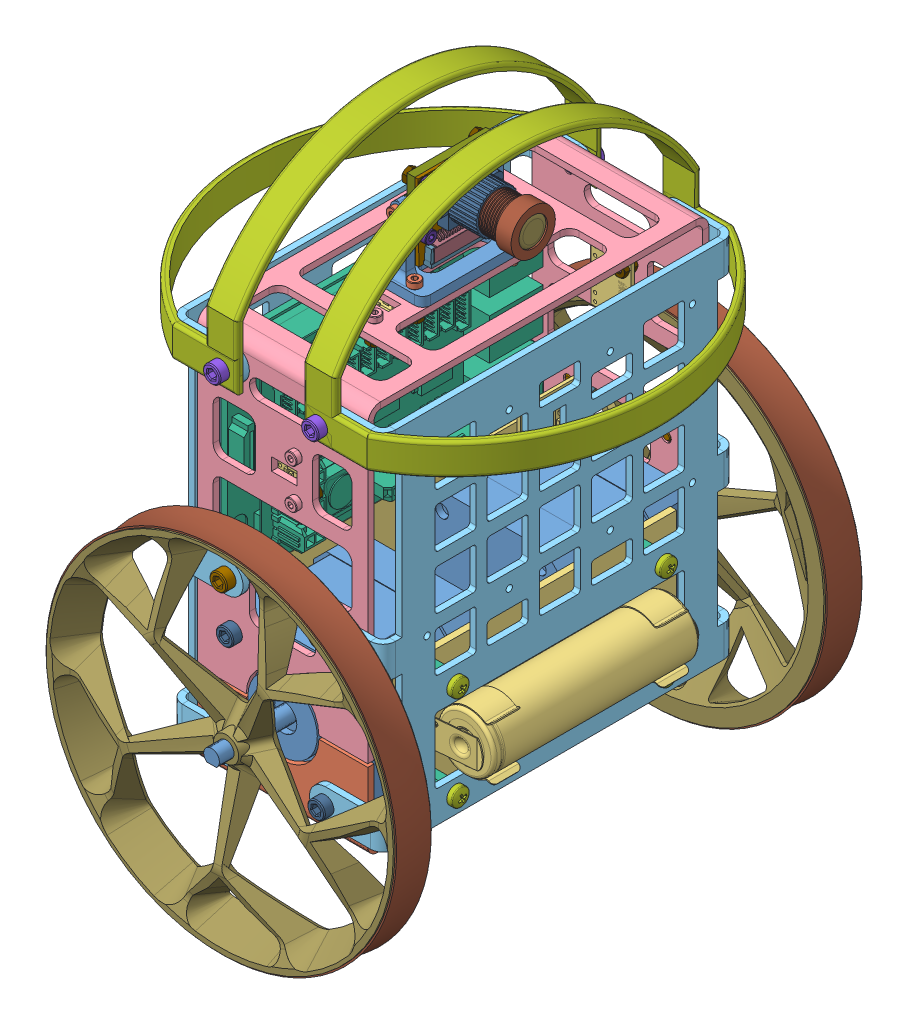
SolidWorks assembly irys4v1, configuration Domyślna. Lengths in mm.
Overall size (135.25 200.37 157.9).
138 component instances, 30 part files, 124 mates.
Components (placement in the parent):
- steppermotor-1: steppermotor [Default] at (-42.2578 -7.1789 72.25) size (42.3 42.3 64.5)
- bottomframe_rys3-1: bottomframe_rys3 [Domyślna] at (-43.1924 -30.5373 18.7182) x (0 0 -1) z (0 -1 0) size (108 54 24.86)
- steppermotor-2: steppermotor [Default] at (-42.2578 -7.1789 -31.75) x (-1 0 0) z (0 0 -1) size (42.3 42.3 64.5)
- battery_module-1: battery_module [Domyślna] at (-62.2578 -30.5373 65.25) x (0 0 -1) z (0 -1 0) size (90 40 22.7)
- topframe-1: topframe [Domyślna] at (-43.6117 88.6087 10.8622) x (0 0 -1) z (0 1 0) size (108 54 97.29)
- front-1: front [Domyślna] at (-74.0454 69.3173 20.0764) x (0 0 1) z (0 -1 0) size (112 23.29 115)
- rys_PCB_rpi_simple-1: rys_PCB_rpi_simple [Domyślna] at (-57.6307 101.7784 107.2123) x (0 -1 0) z (1 0 0) size (61.22 87.74 23.25)
- front-2: front [Domyślna] at (-10.4701 69.3173 20.4236) x (0 0 -1) z (0 -1 0) size (112 23.29 115)
- bumper-2: bumper [Domyślna] at (-72.7578 82.3211 20.318) x (0 0 1) z (0 -1 0) size (116 57.13 10)
- bumper-3: bumper [Domyślna] at (-11.7578 82.3211 20.25) x (0 0 1) z (0 1 0) size (116 57.13 10)
- imu-1: imu [Domyślna] at (-53.5985 -9.4799 25.3181) x (-0.019519 0 -0.999809) z (0 -1 0) size (10.16 22.86 2.23)
- camera_mounted-1: camera_mounted [Domyślna] at (-48.1687 108.7904 16.7906) x (0 0 -1) z (0.999935 0.011413 0) size (36.3 30.27 33.11)
  - Camera Module Assem-1: Camera Module Assem [Default] at (-12.4357 -13.5775 -13.0743) size (25 24 24.98)
    - PCB 1-1: PCB 1 [Default] at (8.9736 12.851 19.5114) size (25 24 2.1)
    - Camera Block-1: Camera Block [Default] at (8.9736 15.851 20.5114) size (22 13.5 12.5)
    - Camera end-1: Camera end [Default] at (8.9736 15.851 27.3922) x (0.999924 0.012337 0) z (0 0 1) size (14 14 17.26)
    - Lenz-1: Lenz [Default] at (8.9736 15.851 43.8922) size (9 9 0.5)
    - 15 Pin Ribbon Block Assem-1: 15 Pin Ribbon Block Assem [Default] at (0.7567 20.5462 10.9417) x (1 0 0) z (0 -1 0) size (22 2.5 7)
      - 15 Pin Ribbon Block-1: 15 Pin Ribbon Block [Default] at (8.217 10.8197 14.6952) size (20 2.5 6)
      - Ribbon Clamp-1: Ribbon Clamp [Default] at (8.217 10.8197 14.6952) size (22 2.5 5)
    - 0603 Resistor-1: 0603 Resistor [Default] at (2.3268 23.572 20.4882) size (1.75 0.89 0.66)
    - 0603 Resistor-2: 0603 Resistor [Default] at (4.5768 23.572 20.4882) size (1.75 0.89 0.66)
    - 0603 Resistor-3: 0603 Resistor [Default] at (15.6203 23.5707 20.4857) size (1.75 0.89 0.66)
    - 0603 Resistor-4: 0603 Resistor [Default] at (13.3703 23.5707 20.4857) size (1.75 0.89 0.66)
  - mount-1: mount [Domyślna] at (-15.8432 -12.9016 1.4371) size (25 24 5)
  - M2 x 0.4mm Thread 5mm LONG SOCKET HEAD CAP SCREW-1: M2 x 0.4mm Thread 5mm LONG SOCKET HEAD CAP SCREW [Domyślna] at (7.0379 9.2735 2.5371) x (-0.356462 0.93431 0) z (0 0 -1) size (3.8 3.8 7.09)
  - M2 x 0.4mm Thread 5mm LONG SOCKET HEAD CAP SCREW-2: M2 x 0.4mm Thread 5mm LONG SOCKET HEAD CAP SCREW [Domyślna] at (7.0379 -4.7265 2.5371) x (-0.994039 0.109029 0) z (0 0 -1) size (3.8 3.8 7.09)
  - M2 x 0.4mm Thread 5mm LONG SOCKET HEAD CAP SCREW-3: M2 x 0.4mm Thread 5mm LONG SOCKET HEAD CAP SCREW [Domyślna] at (-13.9621 9.2735 2.5371) x (-0.583934 -0.811801 0) z (0 0 -1) size (3.8 3.8 7.09)
  - M2 x 0.4mm Thread 5mm LONG SOCKET HEAD CAP SCREW-4: M2 x 0.4mm Thread 5mm LONG SOCKET HEAD CAP SCREW [Domyślna] at (-13.9621 -4.7265 2.5371) x (-0.923728 -0.383049 0) z (0 0 -1) size (3.8 3.8 7.09)
  - m2_x_0_4mm_thread_hex_nut-1: m2_x_0_4mm_thread_hex_nut [Domyślna] at (7.0379 9.2735 3.1371) size (4 4.62 1.6)
  - m2_x_0_4mm_thread_hex_nut-2: m2_x_0_4mm_thread_hex_nut [Domyślna] at (7.0379 -4.7265 3.1371) size (4 4.62 1.6)
  - m2_x_0_4mm_thread_hex_nut-3: m2_x_0_4mm_thread_hex_nut [Domyślna] at (-13.9621 -4.7265 3.1371) size (4 4.62 1.6)
  - m2_x_0_4mm_thread_hex_nut-4: m2_x_0_4mm_thread_hex_nut [Domyślna] at (-13.9621 9.2735 3.1371) size (4 4.62 1.6)
  - mount1-1: mount1 [Domyślna] at (7.7442 -6.03 1.3422) x (1 0 0) z (0 -0.011413 0.999935) size (36.3 23 16)
  - M2 x 0.4mm Thread 10mm LONG SOCKET HEAD CAP SCREW-1: M2 x 0.4mm Thread 10mm LONG SOCKET HEAD CAP SCREW [Domyślna] at (1.9591 2.2735 3.9371) x (0 0.966896 -0.255169) z (-1 0 0) size (3.8 3.8 12.09)
  - M2 x 0.4mm Thread 10mm LONG SOCKET HEAD CAP SCREW-2: M2 x 0.4mm Thread 10mm LONG SOCKET HEAD CAP SCREW [Domyślna] at (-8.8833 2.2735 3.9371) x (0 0 -1) z (1 0 0) size (3.8 3.8 12.09)
- bumper-4: bumper [Domyślna] at (-57.7497 97.3211 20.25) x (0 0 1) z (-1 0.000537 0) size (116 57.13 10)
- bumper-5: bumper [Domyślna] at (-26.7108 97.321 20.25) x (0 0 1) z (-0.999995 0.003129 0) size (116 57.13 10)
- M2 x 0.4mm Thread 10mm LONG SOCKET HEAD CAP SCREW-1: M2 x 0.4mm Thread 10mm LONG SOCKET HEAD CAP SCREW [Domyślna] at (-66.2815 25.7406 61.8682) x (0 -0.924225 -0.381849) z (1 0 0) size (3.8 3.8 12.09)
- M2 x 0.4mm Thread 10mm LONG SOCKET HEAD CAP SCREW-2: M2 x 0.4mm Thread 10mm LONG SOCKET HEAD CAP SCREW [Domyślna] at (-65.9407 73.8539 61.4153) x (0 -0.924225 -0.381849) z (1 0 0) size (3.8 3.8 12.09)
- ToF_nut-3: ToF_nut [Domyślna] at (-29.7647 62.6897 19.6577) x (0 -1 0) z (1 0 0) size (12.89 18.5 4.22)
  - vl53l1x-1: vl53l1x [Domyślna] at (-6.7913 -9.4823 16.6745) size (12.7 17.78 2.22)
  - m2_x_0_4mm_thread_hex_nut-1: m2_x_0_4mm_thread_hex_nut [Domyślna] at (3.3687 5.7577 15.8745) size (4 4.62 1.6)
  - m2_x_0_4mm_thread_hex_nut-2: m2_x_0_4mm_thread_hex_nut [Domyślna] at (3.3687 -6.9423 15.8745) x (-0.923728 -0.383049 0) z (0 0 -1) size (4 4.62 1.6)
  - m2_x_0_4mm_thread_hex_nut-3: m2_x_0_4mm_thread_hex_nut [Domyślna] at (3.3687 5.7577 18.4945) x (-0.923728 -0.383049 0) z (0 0 -1) size (4 4.62 1.6)
  - m2_x_0_4mm_thread_hex_nut-4: m2_x_0_4mm_thread_hex_nut [Domyślna] at (3.3687 -6.9423 18.4945) x (-0.923728 -0.383049 0) z (0 0 -1) size (4 4.62 1.6)
- m2_x_0_4mm_thread_6mm_long_sock-3: m2_x_0_4mm_thread_6mm_long_sock [Domyślna] at (-14.4701 59.3211 13.9) x (0 0.924225 0.381849) z (-1 0 0) size (3.8 3.8 8)
- m2_x_0_4mm_thread_6mm_long_sock-5: m2_x_0_4mm_thread_6mm_long_sock [Domyślna] at (-14.4701 59.3211 26.6) x (0 0.924225 0.381849) z (-1 0 0) size (3.8 3.8 8)
- ToF_nut-5: ToF_nut [Domyślna] at (-42.1264 69.3142 41.6577) x (1 0 0) z (0 1 0) size (12.89 18.5 4.22)
  - vl53l1x-1: vl53l1x [Domyślna] at (-6.7913 -9.4823 16.6745) size (12.7 17.78 2.22)
  - m2_x_0_4mm_thread_hex_nut-1: m2_x_0_4mm_thread_hex_nut [Domyślna] at (3.3687 5.7577 15.8745) size (4 4.62 1.6)
  - m2_x_0_4mm_thread_hex_nut-2: m2_x_0_4mm_thread_hex_nut [Domyślna] at (3.3687 -6.9423 15.8745) x (-0.923728 -0.383049 0) z (0 0 -1) size (4 4.62 1.6)
  - m2_x_0_4mm_thread_hex_nut-3: m2_x_0_4mm_thread_hex_nut [Domyślna] at (3.3687 5.7577 18.4945) x (-0.923728 -0.383049 0) z (0 0 -1) size (4 4.62 1.6)
  - m2_x_0_4mm_thread_hex_nut-4: m2_x_0_4mm_thread_hex_nut [Domyślna] at (3.3687 -6.9423 18.4945) x (-0.923728 -0.383049 0) z (0 0 -1) size (4 4.62 1.6)
- M2 x 0.4mm Thread 10mm LONG SOCKET HEAD CAP SCREW-3: M2 x 0.4mm Thread 10mm LONG SOCKET HEAD CAP SCREW [Domyślna] at (-38.7578 83.6087 4.6) x (0.952226 0 0.305395) z (0 -1 0) size (3.8 3.8 12.09)
- M2 x 0.4mm Thread 10mm LONG SOCKET HEAD CAP SCREW-4: M2 x 0.4mm Thread 10mm LONG SOCKET HEAD CAP SCREW [Domyślna] at (-38.7578 83.6087 35.9) x (0.999568 0 -0.029375) z (0 -1 0) size (3.8 3.8 12.09)
- m2_x_0_4mm_thread_6mm_long_sock-7: m2_x_0_4mm_thread_6mm_long_sock [Domyślna] at (-38.7578 84.6087 48.6) x (-0.868702 0 -0.495335) z (0 -1 0) size (3.8 3.8 8)
- ToF_nut-6: ToF_nut [Domyślna] at (-41.1264 60.9134 52.9555) size (12.89 18.5 4.22)
  - vl53l1x-1: vl53l1x [Domyślna] at (-6.7913 -9.4823 16.6745) size (12.7 17.78 2.22)
  - m2_x_0_4mm_thread_hex_nut-1: m2_x_0_4mm_thread_hex_nut [Domyślna] at (3.3687 5.7577 15.8745) size (4 4.62 1.6)
  - m2_x_0_4mm_thread_hex_nut-2: m2_x_0_4mm_thread_hex_nut [Domyślna] at (3.3687 -6.9423 15.8745) x (-0.923728 -0.383049 0) z (0 0 -1) size (4 4.62 1.6)
  - m2_x_0_4mm_thread_hex_nut-3: m2_x_0_4mm_thread_hex_nut [Domyślna] at (3.3687 5.7577 18.4945) x (-0.923728 -0.383049 0) z (0 0 -1) size (4 4.62 1.6)
  - m2_x_0_4mm_thread_hex_nut-4: m2_x_0_4mm_thread_hex_nut [Domyślna] at (3.3687 -6.9423 18.4945) x (-0.923728 -0.383049 0) z (0 0 -1) size (4 4.62 1.6)
- ToF_nut-7: ToF_nut [Domyślna] at (-41.1264 59.7288 -12.4555) x (1 0 0) z (0 0 -1) size (12.89 18.5 4.22)
  - vl53l1x-1: vl53l1x [Domyślna] at (-6.7913 -9.4823 16.6745) size (12.7 17.78 2.22)
  - m2_x_0_4mm_thread_hex_nut-1: m2_x_0_4mm_thread_hex_nut [Domyślna] at (3.3687 5.7577 15.8745) size (4 4.62 1.6)
  - m2_x_0_4mm_thread_hex_nut-2: m2_x_0_4mm_thread_hex_nut [Domyślna] at (3.3687 -6.9423 15.8745) x (-0.923728 -0.383049 0) z (0 0 -1) size (4 4.62 1.6)
  - m2_x_0_4mm_thread_hex_nut-3: m2_x_0_4mm_thread_hex_nut [Domyślna] at (3.3687 5.7577 18.4945) x (-0.923728 -0.383049 0) z (0 0 -1) size (4 4.62 1.6)
  - m2_x_0_4mm_thread_hex_nut-4: m2_x_0_4mm_thread_hex_nut [Domyślna] at (3.3687 -6.9423 18.4945) x (-0.923728 -0.383049 0) z (0 0 -1) size (4 4.62 1.6)
- ToF_nut-9: ToF_nut [Domyślna] at (-54.7508 62.6897 20.8423) x (0 -1 0) z (-1 0 0) size (12.89 18.5 4.22)
  - vl53l1x-1: vl53l1x [Domyślna] at (-6.7913 -9.4823 16.6745) size (12.7 17.78 2.22)
  - m2_x_0_4mm_thread_hex_nut-1: m2_x_0_4mm_thread_hex_nut [Domyślna] at (3.3687 5.7577 15.8745) size (4 4.62 1.6)
  - m2_x_0_4mm_thread_hex_nut-2: m2_x_0_4mm_thread_hex_nut [Domyślna] at (3.3687 -6.9423 15.8745) x (-0.923728 -0.383049 0) z (0 0 -1) size (4 4.62 1.6)
  - m2_x_0_4mm_thread_hex_nut-3: m2_x_0_4mm_thread_hex_nut [Domyślna] at (3.3687 5.7577 18.4945) x (-0.923728 -0.383049 0) z (0 0 -1) size (4 4.62 1.6)
  - m2_x_0_4mm_thread_hex_nut-4: m2_x_0_4mm_thread_hex_nut [Domyślna] at (3.3687 -6.9423 18.4945) x (-0.923728 -0.383049 0) z (0 0 -1) size (4 4.62 1.6)
- m2_x_0_4mm_thread_6mm_long_sock-11: m2_x_0_4mm_thread_6mm_long_sock [Domyślna] at (-70.0454 59.3211 13.9) x (0 -0.924225 -0.381849) z (1 0 0) size (3.8 3.8 8)
- m2_x_0_4mm_thread_6mm_long_sock-12: m2_x_0_4mm_thread_6mm_long_sock [Domyślna] at (-70.0454 59.3211 26.6) x (0 -0.924225 -0.381849) z (1 0 0) size (3.8 3.8 8)
- m2_x_0_4mm_thread_6mm_long_sock-15: m2_x_0_4mm_thread_6mm_long_sock [Domyślna] at (-37.7578 66.6711 68.25) x (-0.262854 -0.964836 0) z (0 0 -1) size (3.8 3.8 8)
- m2_x_0_4mm_thread_6mm_long_sock-16: m2_x_0_4mm_thread_6mm_long_sock [Domyślna] at (-37.7578 53.9711 68.25) x (0.638921 -0.769272 0) z (0 0 -1) size (3.8 3.8 8)
- m2_x_0_4mm_thread_6mm_long_sock-17: m2_x_0_4mm_thread_6mm_long_sock [Domyślna] at (-37.7578 66.6711 -27.75) size (3.8 3.8 8)
- m2_x_0_4mm_thread_6mm_long_sock-18: m2_x_0_4mm_thread_6mm_long_sock [Domyślna] at (-37.7578 53.9711 -27.75) size (3.8 3.8 8)
- H-H_M3x12mm-1: H-H_M3x12mm [Predeterminado] at (-51.2078 -22.4959 17.65) x (0.837169 0 0.546944) z (0.546944 0 -0.837169) size (5.77 12 5)
- H-H_M3x6mm-1: H-H_M3x6mm [Predeterminado] at (-51.2078 -13.4959 17.65) x (0.837169 0 0.546944) z (0.546944 0 -0.837169) size (5.77 6 5)
- pan cross head_am-2: pan cross head_am [B18.6.7M - M3 x 0.5 x 6 Type I Cross Recessed PHMS --6N] at (-51.2078 -7.0799 17.65) x (0 -1 0) z (0 0 1) size (8.37 5.6 5.6)
- battery_module_H-2: battery_module_H [Domyślna] at (13.655 -6.0808 19.8906) x (0 0 1) z (-1 0 0) size (90 40 24.06)
  - battery_module-1: battery_module [Domyślna] at (-44.6406 -21.0981 81.7004) size (90 40 22.7)
  - H-H_M3x6mm-1: H-H_M3x6mm [Predeterminado] at (-32.6406 13.9019 84.7004) x (1 0 0) z (0 1 0) size (5.77 6 5)
  - H-H_M3x6mm-2: H-H_M3x6mm [Predeterminado] at (33.3594 13.9019 84.7004) x (1 0 0) z (0 1 0) size (5.77 6 5)
  - H-H_M3x6mm-3: H-H_M3x6mm [Predeterminado] at (-32.6406 -16.0981 84.7004) x (1 0 0) z (0 -1 0) size (5.77 6 5)
  - H-H_M3x6mm-4: H-H_M3x6mm [Predeterminado] at (33.3594 -16.0981 84.7004) x (1 0 0) z (0 1 0) size (5.77 6 5)
  - pan cross head_am-1: pan cross head_am [B18.6.7M - M3 x 0.5 x 6 Type I Cross Recessed PHMS --6N] at (-32.6406 -16.0981 77.2589) x (0 0 1) z (-1 0 0) size (8.37 5.6 5.6)
  - pan cross head_am-3: pan cross head_am [B18.6.7M - M3 x 0.5 x 6 Type I Cross Recessed PHMS --6N] at (-32.6406 13.9019 77.2589) x (0 0 1) z (-1 0 0) size (8.37 5.6 5.6)
  - pan cross head_am-4: pan cross head_am [B18.6.7M - M3 x 0.5 x 6 Type I Cross Recessed PHMS --6N] at (33.3594 13.9019 77.2589) x (0 0 1) z (-1 0 0) size (8.37 5.6 5.6)
  - pan cross head_am-5: pan cross head_am [B18.6.7M - M3 x 0.5 x 6 Type I Cross Recessed PHMS --6N] at (33.3594 -16.0981 77.2589) x (0 0 1) z (-1 0 0) size (8.37 5.6 5.6)
- pan cross head_am-3: pan cross head_am [B18.6.7M - M3 x 0.5 x 6 Type I Cross Recessed PHMS --6N] at (-78.4454 -22.1789 53.25) size (8.37 5.6 5.6)
- pan cross head_am-4: pan cross head_am [B18.6.7M - M3 x 0.5 x 6 Type I Cross Recessed PHMS --6N] at (-78.4454 7.8211 53.25) size (8.37 5.6 5.6)
- pan cross head_am-5: pan cross head_am [B18.6.7M - M3 x 0.5 x 6 Type I Cross Recessed PHMS --6N] at (-78.4454 7.8211 -12.75) size (8.37 5.6 5.6)
- pan cross head_am-6: pan cross head_am [B18.6.7M - M3 x 0.5 x 6 Type I Cross Recessed PHMS --6N] at (-78.4454 -22.1789 -12.75) size (8.37 5.6 5.6)
- pan cross head_am-7: pan cross head_am [B18.6.7M - M3 x 0.5 x 6 Type I Cross Recessed PHMS --6N] at (-57.2578 -34.9373 53.25) x (0 1 0) z (0 0 1) size (8.37 5.6 5.6)
- pan cross head_am-8: pan cross head_am [B18.6.7M - M3 x 0.5 x 6 Type I Cross Recessed PHMS --6N] at (-27.2578 -34.9373 53.25) x (0 1 0) z (0 0 1) size (8.37 5.6 5.6)
- pan cross head_am-9: pan cross head_am [B18.6.7M - M3 x 0.5 x 6 Type I Cross Recessed PHMS --6N] at (-57.2578 -34.9373 -12.75) x (0 1 0) z (0 0 1) size (8.37 5.6 5.6)
- pan cross head_am-10: pan cross head_am [B18.6.7M - M3 x 0.5 x 6 Type I Cross Recessed PHMS --6N] at (-27.2578 -34.9373 -12.75) x (0 1 0) z (0 0 1) size (8.37 5.6 5.6)
- battery_module_H-3: battery_module_H [Domyślna] at (-98.1705 -8.277 19.8906) x (0 0 1) z (1 0 0) size (90 40 24.06)
  - battery_module-1: battery_module [Domyślna] at (-44.6406 -21.0981 81.7004) size (90 40 22.7)
  - H-H_M3x6mm-1: H-H_M3x6mm [Predeterminado] at (-32.6406 13.9019 84.7004) x (1 0 0) z (0 1 0) size (5.77 6 5)
  - H-H_M3x6mm-2: H-H_M3x6mm [Predeterminado] at (33.3594 13.9019 84.7004) x (1 0 0) z (0 1 0) size (5.77 6 5)
  - H-H_M3x6mm-3: H-H_M3x6mm [Predeterminado] at (-32.6406 -16.0981 84.7004) x (1 0 0) z (0 -1 0) size (5.77 6 5)
  - H-H_M3x6mm-4: H-H_M3x6mm [Predeterminado] at (33.3594 -16.0981 84.7004) x (1 0 0) z (0 1 0) size (5.77 6 5)
  - pan cross head_am-1: pan cross head_am [B18.6.7M - M3 x 0.5 x 6 Type I Cross Recessed PHMS --6N] at (-32.6406 -16.0981 77.2589) x (0 0 1) z (-1 0 0) size (8.37 5.6 5.6)
  - pan cross head_am-3: pan cross head_am [B18.6.7M - M3 x 0.5 x 6 Type I Cross Recessed PHMS --6N] at (-32.6406 13.9019 77.2589) x (0 0 1) z (-1 0 0) size (8.37 5.6 5.6)
  - pan cross head_am-4: pan cross head_am [B18.6.7M - M3 x 0.5 x 6 Type I Cross Recessed PHMS --6N] at (33.3594 13.9019 77.2589) x (0 0 1) z (-1 0 0) size (8.37 5.6 5.6)
  - pan cross head_am-5: pan cross head_am [B18.6.7M - M3 x 0.5 x 6 Type I Cross Recessed PHMS --6N] at (33.3594 -16.0981 77.2589) x (0 0 1) z (-1 0 0) size (8.37 5.6 5.6)
- pan cross head_am-11: pan cross head_am [B18.6.7M - M3 x 0.5 x 6 Type I Cross Recessed PHMS --6N] at (-6.0701 -22.1789 53.25) x (-1 0 0) z (0 0.924225 0.381849) size (8.37 5.6 5.6)
- pan cross head_am-12: pan cross head_am [B18.6.7M - M3 x 0.5 x 6 Type I Cross Recessed PHMS --6N] at (-6.0701 7.8211 53.25) x (-1 0 0) z (0 0.924225 0.381849) size (8.37 5.6 5.6)
- pan cross head_am-13: pan cross head_am [B18.6.7M - M3 x 0.5 x 6 Type I Cross Recessed PHMS --6N] at (-6.0701 7.8211 -12.75) x (-1 0 0) z (0 0.924225 0.381849) size (8.37 5.6 5.6)
- pan cross head_am-14: pan cross head_am [B18.6.7M - M3 x 0.5 x 6 Type I Cross Recessed PHMS --6N] at (-6.0701 -22.1789 -12.75) x (-1 0 0) z (0 0.924225 0.381849) size (8.37 5.6 5.6)
- M3x6-1: M3x6 [Default] at (-57.7578 82.3211 -40.75) x (0 0 1) z (0.923728 0.383049 0) size (9 5.5 5.5)
- M3x6-2: M3x6 [Default] at (-26.7578 82.3211 -40.75) x (0 0 1) z (0.923728 0.383049 0) size (9 5.5 5.5)
- M3x4-1: M3x4 [Default] at (-26.7578 24.3211 -38.75) x (0 0 1) z (0.923728 0.383049 0) size (7 5.5 5.5)
- M3x4-2: M3x4 [Default] at (-57.7578 24.3211 -38.75) x (0 0 1) z (0.923728 0.383049 0) size (7 5.5 5.5)
- M3x8-1: M3x8 [Default] at (-26.7578 8.3211 -36.75) x (0 0 1) z (0.923728 0.383049 0) size (9 5.5 5.5)
- M3x8-2: M3x8 [Default] at (-57.7578 8.3211 -36.75) x (0 0 1) z (0.923728 0.383049 0) size (9 5.5 5.5)
- M3x8-3: M3x8 [Default] at (-26.7578 -22.6789 -38.75) x (0 0 1) z (-0.923728 -0.383049 0) size (9 5.5 5.5)
- M3x8-4: M3x8 [Default] at (-57.7578 -22.6789 -38.75) x (0 0 1) z (0.923728 0.383049 0) size (9 5.5 5.5)
- M3x6-3: M3x6 [Default] at (-57.7578 82.3211 81.318) x (0 0 -1) z (-0.923728 -0.383049 0) size (9 5.5 5.5)
- M3x6-4: M3x6 [Default] at (-26.7578 82.3211 81.25) x (0 0 -1) z (-0.923728 -0.383049 0) size (9 5.5 5.5)
- M3x4-3: M3x4 [Default] at (-57.7578 24.3211 79.25) x (0 0 -1) z (-0.923728 -0.383049 0) size (7 5.5 5.5)
- M3x4-4: M3x4 [Default] at (-26.7578 24.3211 79.25) x (0 0 -1) z (-0.923728 -0.383049 0) size (7 5.5 5.5)
- M3x8-5: M3x8 [Default] at (-57.7578 8.3211 77.25) x (0 0 -1) z (-0.923728 -0.383049 0) size (9 5.5 5.5)
- M3x8-6: M3x8 [Default] at (-26.7578 8.3211 77.25) x (0 0 -1) z (-0.923728 -0.383049 0) size (9 5.5 5.5)
- M3x8-7: M3x8 [Default] at (-57.7578 -22.6789 79.25) x (0 0 -1) z (-0.923728 -0.383049 0) size (9 5.5 5.5)
- M3x8-8: M3x8 [Default] at (-26.7578 -22.6789 79.25) x (0 0 -1) z (-0.923728 -0.383049 0) size (9 5.5 5.5)
- wheel_module-1: wheel_module [Domyślna] at (-153.2578 -13.8345 -57.8785) x (0 0 1) z (1 0 0) size (16.77 112.94 112.94)
  - tire wide-1: tire wide [Domyślna] at (-0.6464 -6.6556 111) size (11 111 111)
  - wheel_rim_minirys-1: wheel_rim_minirys [Domyślna] at (15.6603 -6.6556 111) x (0 0.027139 0.999632) z (-1 0 0) size (110 110 16.77)
- wheel_module-2: wheel_module [Domyślna] at (-153.4368 -5.0545 97.8035) x (0 0 -1) z (0.999168 0.040772 0) size (16.77 112.94 112.94)
  - tire wide-1: tire wide [Domyślna] at (-0.6464 -6.6556 111) size (11 111 111)
  - wheel_rim_minirys-1: wheel_rim_minirys [Domyślna] at (15.6603 -6.6556 111) x (0 0.027139 0.999632) z (-1 0 0) size (110 110 16.77)
Mates (geometry in assembly coordinates):
- Koncentryczne1: concentric aligned: cylinder of steppermotor-1 through (-26.7578 -22.6789 64.75) axis (0 0 1) radius 1.25; cylinder of bottomframe_rys3-1 through (-26.7578 -22.6789 74.25) axis (0 0 1) radius 1.6
- Koncentryczne2: concentric aligned: cylinder of steppermotor-1 through (-57.7578 -22.6789 64.75) axis (0 0 1) radius 1.25; cylinder of bottomframe_rys3-1 through (-57.7578 -22.6789 74.25) axis (0 0 1) radius 1.6
- Wspólnie1: coincident anti-aligned: plane of steppermotor-1 through (-64.2538 -29.1749 72.25) normal (0 0 1); plane of bottomframe_rys3-1 through (-42.2578 -7.6789 72.25) normal (0 0 -1)
- Koncentryczne3: concentric aligned: cylinder of bottomframe_rys3-1 through (-57.7578 -22.6789 -33.75) axis (0 0 -1) radius 1.6; cylinder of steppermotor-2 through (-57.7578 -22.6789 -24.25) axis (0 0 -1) radius 1.25
- Koncentryczne4: concentric aligned: circle of bottomframe_rys3-1; cylinder of steppermotor-2 through (-26.7578 -22.6789 -24.25) axis (0 0 -1) radius 1.25
- Wspólnie2: coincident anti-aligned: plane of bottomframe_rys3-1 through (-42.2578 -159.6789 -31.75) normal (0 0 1); plane of steppermotor-2 through (-20.2618 -29.1749 -31.75) normal (0 0 -1)
- Koncentryczne7: concentric aligned: cylinder of steppermotor-2 through (-26.7578 8.3211 -24.25) axis (0 0 -1) radius 1.25; cylinder of topframe-1 through (-26.7578 8.3211 -33.75) axis (0 0 -1) radius 1.6
- Koncentryczne8: concentric aligned: cylinder of steppermotor-1 through (-57.7578 8.3211 64.75) axis (0 0 1) radius 1.25; cylinder of topframe-1 through (-57.7578 8.3211 74.25) axis (0 0 1) radius 1.6
- Wspólnie4: coincident anti-aligned: plane of steppermotor-1 through (-64.2538 -29.1749 72.25) normal (0 0 1); plane of topframe-1 through (-42.2578 289.3211 72.25) normal (0 0 -1)
- Koncentryczne9: concentric aligned: cylinder of bottomframe_rys3-1 through (-57.7578 -22.6789 74.25) axis (0 0 1) radius 1.6; cylinder of front-1 through (-57.7578 -22.6789 74.25) axis (0 0 1) radius 1.75
- Koncentryczne10: concentric aligned: cylinder of topframe-1 through (-57.7578 82.3211 74.25) axis (0 0 1) radius 1.4; cylinder of front-1 through (-57.7578 82.3211 74.25) axis (0 0 1) radius 1.75
- Koncentryczne11: concentric aligned: cylinder of topframe-1 through (-57.7578 24.3211 -33.75) axis (0 0 -1) radius 1.6; cylinder of front-1 through (-57.7578 24.3211 -33.75) axis (0 0 -1) radius 1.75
- Wspólnie5: coincident anti-aligned: plane of topframe-1 through (-42.2578 -6.6789 -33.75) normal (0 0 -1); plane of front-1 through (-57.7578 82.3211 -33.75) normal (0 0 1)
- Równolegle2: parallel anti-aligned: plane of topframe-1 through (-42.2578 88.6087 -127.75) normal (0 -1 0); plane of rys_PCB_rpi_simple-1 through (-70.9307 77.2185 65.0473) normal (0 1 0)
- Koncentryczne17: concentric aligned: cylinder of topframe-1 through (-26.7578 24.3211 -33.75) axis (0 0 -1) radius 1.6; cylinder of front-2 through (-26.7578 24.3211 -33.75) axis (0 0 -1) radius 1.75
- Koncentryczne18: concentric aligned: cylinder of bottomframe_rys3-1 through (-26.7578 -22.6789 -33.75) axis (0 0 -1) radius 1.6; cylinder of steppermotor-2 through (-26.7578 -22.6789 -24.25) axis (0 0 -1) radius 1.25
- Wspólnie8: coincident anti-aligned: plane of topframe-1 through (-42.2578 289.3211 74.25) normal (0 0 1); plane of front-2 through (-26.7578 82.3211 74.25) normal (0 0 -1)
- Koncentryczne19: concentric aligned: cylinder of bottomframe_rys3-1 through (-26.7578 -22.6789 74.25) axis (0 0 1) radius 1.6; cylinder of front-2 through (-26.7578 -22.6789 74.25) axis (0 0 1) radius 1.75
- Koncentryczne36: concentric aligned: cylinder of topframe-1 through (-57.7578 82.3211 74.25) axis (0 0 1) radius 1.4; cylinder of bumper-2 through (-57.7578 82.3211 -37.682) axis (0 0 1) radius 1.5
- Koncentryczne37: concentric aligned: cylinder of topframe-1 through (-26.7578 82.3211 74.25) axis (0 0 1) radius 1.4; cylinder of bumper-3 through (-26.7578 82.3211 -37.75) axis (0 0 1) radius 1.5
- Wspólnie17: coincident anti-aligned: plane of front-2 through (115.2422 82.3211 -35.75) normal (0 0 -1); plane of bumper-3 through (-31.7578 77.3211 -35.75) normal (0 0 1)
- Koncentryczne55: concentric aligned: cylinder of battery_module-1 through (-51.2078 -28.4959 17.65) axis (0 1 0) radius 1.1; cylinder of imu-1 through (-51.2078 -10.4959 17.65) axis (0 1 0) radius 1.0922
- Koncentryczne56: concentric anti-aligned: cylinder of bottomframe_rys3-1 through (-27.2578 -32.5373 53.25) axis (0 -1 0) radius 1.4; cylinder of battery_module-1 through (-27.2578 -28.4959 53.25) axis (0 1 0) radius 1.6
- Koncentryczne57: concentric anti-aligned: cylinder of bottomframe_rys3-1 through (-57.2578 -32.5373 -12.75) axis (0 -1 0) radius 1.4; cylinder of battery_module-1 through (-57.2578 -28.4959 -12.75) axis (0 1 0) radius 1.6
- Wspólnie27: coincident anti-aligned: plane of bottomframe_rys3-1 through (-42.2578 -30.5373 96.25) normal (0 1 0); plane of battery_module-1 through (-62.2578 -30.5373 65.25) normal (0 -1 0)
- Koncentryczne63: concentric aligned: cylinder of topframe-1 through (-38.7578 90.6087 4.6) axis (0 1 0) radius 1.25; cylinder of camera_mounted-1/mount1-1 through (-38.7578 90.6087 4.6) axis (0 1 0) radius 1.05
- Koncentryczne65: concentric aligned: cylinder of topframe-1 through (-38.7578 90.6087 35.9) axis (0 1 0) radius 1.25; cylinder of camera_mounted-1/mount1-1 through (-38.7578 90.6087 35.9) axis (0 1 0) radius 1.05
- Koncentryczne66: concentric aligned: cylinder of bumper-2 through (-57.7578 82.3211 -37.682) axis (0 0 1) radius 1.5; cylinder of bumper-4 through (-57.7578 82.3211 -37.75) axis (0 0 1) radius 1.5
- Wspólnie32: coincident: line of front-1 through (-57.7578 77.3211 -35.75) axis (-1 0 0); plane of bumper-4 through (-52.7604 77.3184 -35.75) normal (0 0 1)
- Koncentryczne67: concentric aligned: cylinder of bumper-3 through (-26.7578 82.3211 -37.75) axis (0 0 1) radius 1.5; cylinder of bumper-5 through (-26.7578 82.3211 -37.75) axis (0 0 1) radius 1.5
- Wspólnie33: coincident: line of front-2 through (-26.7578 87.3211 -35.75) axis (1 0 0); plane of bumper-5 through (-21.7734 77.3055 -35.75) normal (0 0 1)
- Wspólnie34: coincident anti-aligned: plane of topframe-1 through (-42.2578 90.6087 -127.75) normal (0 1 0); plane of camera_mounted-1/mount1-1 through (-41.7578 90.6087 2.1027) normal (0 -1 0)
- Koncentryczne86: concentric aligned: cylinder of front-2 through (-10.4701 59.3211 26.6) axis (1 0 0) radius 1.25; cylinder of ToF_nut-3/m2_x_0_4mm_thread_hex_nut-4 through (-10.4701 59.3211 26.6) axis (1 0 0) radius 0.7402
- Koncentryczne87: concentric aligned: cylinder of front-2 through (-10.4701 59.3211 13.9) axis (1 0 0) radius 1.25; cylinder of ToF_nut-3/m2_x_0_4mm_thread_hex_nut-3 through (-10.4701 59.3211 13.9) axis (1 0 0) radius 0.7402
- Koncentryczne94: concentric aligned: cylinder of front-2 through (-10.4701 59.3211 13.9) axis (1 0 0) radius 1.25; cylinder of m2_x_0_4mm_thread_6mm_long_sock-3 through (-6.4701 59.3211 13.9) axis (1 0 0) radius 1.9
- Koncentryczne95: concentric aligned: cylinder of front-2 through (-10.4701 59.3211 26.6) axis (1 0 0) radius 1.25; cylinder of m2_x_0_4mm_thread_6mm_long_sock-5 through (-6.4701 59.3211 26.6) axis (1 0 0) radius 1.9
- Koncentryczne98: concentric aligned: cylinder of topframe-1 through (-38.7578 90.6087 48.6) axis (0 1 0) radius 1.25; cylinder of ToF_nut-5/m2_x_0_4mm_thread_hex_nut-4 through (-38.7578 88.6087 48.6) axis (0 1 0) radius 0.7402
- Koncentryczne99: concentric aligned: cylinder of camera_mounted-1/mount1-1 through (-38.7578 90.6087 35.9) axis (0 1 0) radius 1.05; cylinder of ToF_nut-5/m2_x_0_4mm_thread_hex_nut-3 through (-38.7578 88.6087 35.9) axis (0 1 0) radius 0.7402
- Wspólnie61: coincident anti-aligned: plane of topframe-1 through (-42.2578 88.6087 -127.75) normal (0 -1 0); plane of ToF_nut-5/m2_x_0_4mm_thread_hex_nut-4 through (-37.3526 88.6087 46.7673) normal (0 1 0)
- Koncentryczne100: concentric anti-aligned: cylinder of camera_mounted-1/mount1-1 through (-38.7578 90.6087 35.9) axis (0 1 0) radius 1.05; cylinder of M2 x 0.4mm Thread 10mm LONG SOCKET HEAD CAP SCREW-4 through (-38.7578 95.6087 35.9) axis (0 -1 0) radius 1.9
- Koncentryczne102: concentric anti-aligned: cylinder of camera_mounted-1/mount1-1 through (-38.7578 90.6087 4.6) axis (0 1 0) radius 1.05; cylinder of M2 x 0.4mm Thread 10mm LONG SOCKET HEAD CAP SCREW-3 through (-38.7578 95.6087 4.6) axis (0 -1 0) radius 1.9
- Wspólnie62: coincident anti-aligned: plane of camera_mounted-1/mount1-1 through (-41.7578 93.6087 7.7527) normal (0 1 0); plane of M2 x 0.4mm Thread 10mm LONG SOCKET HEAD CAP SCREW-3 through (-38.7578 93.6087 4.6) normal (0 -1 0)
- Wspólnie64: coincident anti-aligned: plane of camera_mounted-1/mount1-1 through (-41.7578 93.6087 7.7527) normal (0 1 0); plane of M2 x 0.4mm Thread 10mm LONG SOCKET HEAD CAP SCREW-4 through (-38.7578 93.6087 35.9) normal (0 -1 0)
- Koncentryczne104: concentric aligned: cylinder of topframe-1 through (-38.7578 90.6087 48.6) axis (0 1 0) radius 1.25; cylinder of m2_x_0_4mm_thread_6mm_long_sock-7 through (-38.7578 92.6087 48.6) axis (0 1 0) radius 1.9
- Wspólnie65: coincident anti-aligned: plane of topframe-1 through (-42.2578 90.6087 -127.75) normal (0 1 0); plane of m2_x_0_4mm_thread_6mm_long_sock-7 through (-38.7578 90.6087 48.6) normal (0 -1 0)
- Koncentryczne105: concentric anti-aligned: cylinder of topframe-1 through (-37.7578 66.6711 74.25) axis (0 0 1) radius 1.25; cylinder of ToF_nut-6/m2_x_0_4mm_thread_hex_nut-3 through (-37.7578 66.6711 70.65) axis (0 0 -1) radius 1
- Koncentryczne106: concentric aligned: cylinder of topframe-1 through (-37.7578 53.9711 74.25) axis (0 0 1) radius 1.25; cylinder of ToF_nut-6/m2_x_0_4mm_thread_hex_nut-4 through (-37.7578 53.9711 72.25) axis (0 0 1) radius 0.7402
- Wspólnie67: coincident anti-aligned: plane of topframe-1 through (-42.2578 289.3211 72.25) normal (0 0 -1); plane of ToF_nut-6/m2_x_0_4mm_thread_hex_nut-4 through (-36.3526 55.8038 72.25) normal (0 0 1)
- Koncentryczne107: concentric anti-aligned: cylinder of topframe-1 through (-37.7578 53.9711 -33.75) axis (0 0 -1) radius 1.25; cylinder of ToF_nut-7/vl53l1x-1 through (-37.7578 53.9711 -30.15) axis (0 0 1) radius 1.0922
- Koncentryczne108: concentric aligned: cylinder of topframe-1 through (-37.7578 66.6711 -33.75) axis (0 0 -1) radius 1.25; cylinder of ToF_nut-7/m2_x_0_4mm_thread_hex_nut-4 through (-37.7578 66.6711 -31.75) axis (0 0 -1) radius 0.7402
- Wspólnie68: coincident anti-aligned: plane of topframe-1 through (-42.2578 -6.6789 -31.75) normal (0 0 1); plane of ToF_nut-7/m2_x_0_4mm_thread_hex_nut-3 through (-36.3526 52.1384 -31.75) normal (0 0 -1)
- Koncentryczne111: concentric aligned: cylinder of front-1 through (-74.0454 59.3211 13.9) axis (-1 0 0) radius 1.25; cylinder of ToF_nut-9/m2_x_0_4mm_thread_hex_nut-4 through (-74.0454 59.3211 13.9) axis (-1 0 0) radius 0.7402
- Koncentryczne112: concentric aligned: cylinder of front-1 through (-74.0454 59.3211 26.6) axis (-1 0 0) radius 1.25; cylinder of ToF_nut-9/m2_x_0_4mm_thread_hex_nut-3 through (-74.0454 59.3211 26.6) axis (-1 0 0) radius 0.7402
- Koncentryczne117: concentric aligned: cylinder of front-1 through (-74.0454 59.3211 13.9) axis (-1 0 0) radius 1.25; cylinder of m2_x_0_4mm_thread_6mm_long_sock-11 through (-78.0454 59.3211 13.9) axis (-1 0 0) radius 1.9
- Koncentryczne118: concentric aligned: cylinder of front-1 through (-74.0454 59.3211 26.6) axis (-1 0 0) radius 1.25; cylinder of m2_x_0_4mm_thread_6mm_long_sock-12 through (-78.0454 59.3211 26.6) axis (-1 0 0) radius 1.9
- Koncentryczne121: concentric aligned: cylinder of topframe-1 through (-37.7578 53.9711 74.25) axis (0 0 1) radius 1.25; cylinder of m2_x_0_4mm_thread_6mm_long_sock-16 through (-37.7578 53.9711 76.25) axis (0 0 1) radius 1.9
- Koncentryczne122: concentric aligned: cylinder of topframe-1 through (-37.7578 66.6711 74.25) axis (0 0 1) radius 1.25; cylinder of m2_x_0_4mm_thread_6mm_long_sock-15 through (-37.7578 66.6711 76.25) axis (0 0 1) radius 1.9
- Wspólnie78: coincident anti-aligned: plane of topframe-1 through (-42.2578 289.3211 74.25) normal (0 0 1); plane of m2_x_0_4mm_thread_6mm_long_sock-15 through (-37.7578 66.6711 74.25) normal (0 0 -1)
- Wspólnie79: coincident anti-aligned: plane of topframe-1 through (-42.2578 289.3211 74.25) normal (0 0 1); plane of m2_x_0_4mm_thread_6mm_long_sock-16 through (-37.7578 53.9711 74.25) normal (0 0 -1)
- Koncentryczne123: concentric aligned: cylinder of topframe-1 through (-37.7578 53.9711 -33.75) axis (0 0 -1) radius 1.25; cylinder of m2_x_0_4mm_thread_6mm_long_sock-18 through (-37.7578 53.9711 -35.75) axis (0 0 -1) radius 1.9
- Koncentryczne124: concentric aligned: cylinder of topframe-1 through (-37.7578 66.6711 -33.75) axis (0 0 -1) radius 1.25; cylinder of m2_x_0_4mm_thread_6mm_long_sock-17 through (-37.7578 66.6711 -35.75) axis (0 0 -1) radius 1.9
- Wspólnie80: coincident anti-aligned: plane of topframe-1 through (-42.2578 -6.6789 -33.75) normal (0 0 -1); plane of m2_x_0_4mm_thread_6mm_long_sock-17 through (-37.7578 66.6711 -33.75) normal (0 0 1)
- Wspólnie81: coincident anti-aligned: plane of topframe-1 through (-42.2578 -6.6789 -33.75) normal (0 0 -1); plane of m2_x_0_4mm_thread_6mm_long_sock-18 through (-37.7578 53.9711 -33.75) normal (0 0 1)
- Koncentryczne125: concentric aligned: cylinder of battery_module-1 through (-51.2078 -28.4959 17.65) axis (0 1 0) radius 1.1; cylinder of H-H_M3x12mm-1 through (-51.2078 -28.4959 17.65) axis (0 1 0) radius 1.5
- Wspólnie82: coincident anti-aligned: plane of battery_module-1 through (-62.2578 -28.4959 65.25) normal (0 1 0); plane of H-H_M3x12mm-1 through (-51.2078 -28.4959 17.65) normal (0 -1 0)
- Wspólnie83: coincident anti-aligned: circle of H-H_M3x12mm-1; cylinder of H-H_M3x6mm-1 through (-51.2078 -16.4959 17.65) axis (0 1 0) radius 1.5
- Wspólnie84: coincident anti-aligned: plane of H-H_M3x12mm-1 through (-51.2078 -16.4959 17.65) normal (0 1 0); plane of H-H_M3x6mm-1 through (-51.2078 -16.4959 17.65) normal (0 -1 0)
- Wspólnie85: coincident anti-aligned: plane of imu-1 through (-53.5985 -10.4959 25.3181) normal (0 -1 0); plane of H-H_M3x6mm-1 through (-51.2078 -10.4959 17.65) normal (0 1 0)
- Koncentryczne1261: concentric aligned: cylinder of imu-1 through (-51.2078 -10.4959 17.65) axis (0 1 0) radius 1.0922; cylinder of pan cross head_am-2 through (-51.2078 18.3201 17.65) axis (0 1 0) radius 2.8
- Wspólnie871: coincident anti-aligned: plane of imu-1 through (-53.5985 -9.4799 25.3181) normal (0 1 0); plane of pan cross head_am-2 through (-49.7078 -9.4799 17.65) normal (0 -1 0)
- Koncentryczne127: concentric aligned: cylinder of front-1 through (-74.0454 7.8211 -12.75) axis (-1 0 0) radius 1.4; cylinder of battery_module_H-2/H-H_M3x6mm-1 through (-68.0454 7.8211 -12.75) axis (-1 0 0) radius 1.5
- Koncentryczne128: concentric aligned: cylinder of front-1 through (-74.0454 -22.1789 53.25) axis (-1 0 0) radius 1.4; cylinder of battery_module_H-2/H-H_M3x6mm-4 through (-68.0454 -22.1789 53.25) axis (-1 0 0) radius 1.5
- Koncentryczne1291: concentric aligned: cylinder of front-1 through (-74.0454 -22.1789 53.25) axis (-1 0 0) radius 1.4; cylinder of pan cross head_am-3 through (-103.8454 -22.1789 53.25) axis (-1 0 0) radius 2.8
- Koncentryczne1301: concentric aligned: cylinder of front-1 through (-74.0454 7.8211 53.25) axis (-1 0 0) radius 1.4; cylinder of pan cross head_am-4 through (-103.8454 7.8211 53.25) axis (-1 0 0) radius 2.8
- Koncentryczne1311: concentric aligned: cylinder of front-1 through (-74.0454 7.8211 -12.75) axis (-1 0 0) radius 1.4; cylinder of pan cross head_am-5 through (-103.8454 7.8211 -12.75) axis (-1 0 0) radius 2.8
- Koncentryczne1321: concentric aligned: cylinder of front-1 through (-74.0454 -22.1789 -12.75) axis (-1 0 0) radius 1.4; cylinder of pan cross head_am-6 through (-103.8454 -22.1789 -12.75) axis (-1 0 0) radius 2.8
- Koncentryczne1331: concentric aligned: cylinder of bottomframe_rys3-1 through (-57.2578 -32.5373 53.25) axis (0 -1 0) radius 1.4; cylinder of pan cross head_am-7 through (-57.2578 -60.3373 53.25) axis (0 -1 0) radius 2.8
- Wspólnie931: coincident anti-aligned: plane of bottomframe_rys3-1 through (-42.2578 -32.5373 96.25) normal (0 -1 0); plane of pan cross head_am-7 through (-58.7578 -32.5373 53.25) normal (0 1 0)
- Koncentryczne1341: concentric aligned: cylinder of bottomframe_rys3-1 through (-27.2578 -32.5373 53.25) axis (0 -1 0) radius 1.4; cylinder of pan cross head_am-8 through (-27.2578 -60.3373 53.25) axis (0 -1 0) radius 2.8
- Wspólnie941: coincident anti-aligned: plane of bottomframe_rys3-1 through (-42.2578 -32.5373 96.25) normal (0 -1 0); plane of pan cross head_am-8 through (-28.7578 -32.5373 53.25) normal (0 1 0)
- Koncentryczne1351: concentric aligned: cylinder of bottomframe_rys3-1 through (-57.2578 -32.5373 -12.75) axis (0 -1 0) radius 1.4; cylinder of pan cross head_am-9 through (-57.2578 -60.3373 -12.75) axis (0 -1 0) radius 2.8
- Wspólnie951: coincident anti-aligned: plane of bottomframe_rys3-1 through (-42.2578 -32.5373 96.25) normal (0 -1 0); plane of pan cross head_am-9 through (-58.7578 -32.5373 -12.75) normal (0 1 0)
- Koncentryczne1361: concentric aligned: cylinder of bottomframe_rys3-1 through (-27.2578 -32.5373 -12.75) axis (0 -1 0) radius 1.4; cylinder of pan cross head_am-10 through (-27.2578 -60.3373 -12.75) axis (0 -1 0) radius 2.8
- Wspólnie961: coincident anti-aligned: plane of bottomframe_rys3-1 through (-42.2578 -32.5373 96.25) normal (0 -1 0); plane of pan cross head_am-10 through (-28.7578 -32.5373 -12.75) normal (0 1 0)
- Koncentryczne138: concentric aligned: cylinder of front-2 through (-10.4701 -22.1789 -12.75) axis (1 0 0) radius 1.4; cylinder of battery_module_H-3/H-H_M3x6mm-1 through (-16.4701 -22.1789 -12.75) axis (1 0 0) radius 1.5
- Koncentryczne139: concentric aligned: cylinder of front-2 through (-10.4701 7.8211 53.25) axis (1 0 0) radius 1.4; cylinder of battery_module_H-3/H-H_M3x6mm-4 through (-16.4701 7.8211 53.25) axis (1 0 0) radius 1.5
- Koncentryczne1401: concentric aligned: cylinder of front-2 through (-10.4701 -22.1789 53.25) axis (1 0 0) radius 1.4; cylinder of pan cross head_am-11 through (19.3299 -22.1789 53.25) axis (1 0 0) radius 2.8
- Koncentryczne1411: concentric aligned: cylinder of front-2 through (-10.4701 7.8211 53.25) axis (1 0 0) radius 1.4; cylinder of pan cross head_am-12 through (19.3299 7.8211 53.25) axis (1 0 0) radius 2.8
- Koncentryczne1421: concentric aligned: cylinder of front-2 through (-10.4701 7.8211 -12.75) axis (1 0 0) radius 1.4; cylinder of pan cross head_am-13 through (19.3299 7.8211 -12.75) axis (1 0 0) radius 2.8
- Koncentryczne1431: concentric aligned: cylinder of front-2 through (-10.4701 -22.1789 -12.75) axis (1 0 0) radius 1.4; cylinder of pan cross head_am-14 through (19.3299 -22.1789 -12.75) axis (1 0 0) radius 2.8
- Koncentryczne144: concentric aligned: cylinder of front-1 through (-57.7578 82.3211 -33.75) axis (0 0 -1) radius 1.75; cylinder of M3x6-1 through (-57.7578 82.3211 -129.4555) axis (0 0 -1) radius 2.75
- Wspólnie103: coincident anti-aligned: plane of bumper-4 through (-52.7604 77.3184 -37.75) normal (0 0 -1); plane of M3x6-1 through (-57.187 80.9447 -37.75) normal (0 0 1)
- Koncentryczne145: concentric aligned: cylinder of front-2 through (-26.7578 82.3211 -33.75) axis (0 0 -1) radius 1.75; cylinder of M3x6-2 through (-26.7578 82.3211 -129.4555) axis (0 0 -1) radius 2.75
- Wspólnie104: coincident anti-aligned: plane of bumper-3 through (-31.7578 77.3211 -37.75) normal (0 0 -1); plane of M3x6-2 through (-26.187 80.9447 -37.75) normal (0 0 1)
- Koncentryczne146: concentric aligned: cylinder of front-2 through (-26.7578 24.3211 -33.75) axis (0 0 -1) radius 1.75; cylinder of M3x4-1 through (-26.7578 24.3211 -127.4555) axis (0 0 -1) radius 2.75
- Koncentryczne147: concentric aligned: cylinder of front-1 through (-57.7578 24.3211 -33.75) axis (0 0 -1) radius 1.75; cylinder of M3x4-2 through (-57.7578 24.3211 -127.4555) axis (0 0 -1) radius 2.75
- Wspólnie105: coincident anti-aligned: plane of front-1 through (-57.7578 82.3211 -35.75) normal (0 0 -1); plane of M3x4-2 through (-57.187 22.9447 -35.75) normal (0 0 1)
- Wspólnie106: coincident anti-aligned: plane of front-2 through (115.2422 82.3211 -35.75) normal (0 0 -1); plane of M3x4-1 through (-26.187 22.9447 -35.75) normal (0 0 1)
- Koncentryczne148: concentric aligned: cylinder of topframe-1 through (-26.7578 8.3211 -33.75) axis (0 0 -1) radius 1.6; cylinder of M3x8-1 through (-26.7578 8.3211 -125.4555) axis (0 0 -1) radius 2.75
- Wspólnie107: coincident anti-aligned: plane of topframe-1 through (-42.2578 -6.6789 -33.75) normal (0 0 -1); plane of M3x8-1 through (-26.187 6.9447 -33.75) normal (0 0 1)
- Koncentryczne149: concentric aligned: cylinder of topframe-1 through (-57.7578 8.3211 -33.75) axis (0 0 -1) radius 1.6; cylinder of M3x8-2 through (-57.7578 8.3211 -125.4555) axis (0 0 -1) radius 2.75
- Wspólnie108: coincident anti-aligned: plane of topframe-1 through (-42.2578 -6.6789 -33.75) normal (0 0 -1); plane of M3x8-2 through (-57.187 6.9447 -33.75) normal (0 0 1)
- Koncentryczne150: concentric aligned: cylinder of bottomframe_rys3-1 through (-57.7578 -22.6789 -33.75) axis (0 0 -1) radius 1.6; cylinder of M3x8-4 through (-57.7578 -22.6789 -127.4555) axis (0 0 -1) radius 2.75
- Koncentryczne151: concentric aligned: cylinder of front-2 through (-26.7578 -22.6789 -33.75) axis (0 0 -1) radius 1.75; cylinder of M3x8-3 through (-26.7578 -22.6789 -127.4555) axis (0 0 -1) radius 2.75
- Wspólnie109: coincident anti-aligned: plane of front-1 through (-57.7578 82.3211 -35.75) normal (0 0 -1); plane of M3x8-4 through (-57.187 -24.0553 -35.75) normal (0 0 1)
- Wspólnie110: coincident aligned: plane of front-2 through (115.2422 82.3211 -35.75) normal (0 0 -1); circle of M3x8-3
- Koncentryczne152: concentric aligned: cylinder of front-2 through (-26.7578 82.3211 74.25) axis (0 0 1) radius 1.75; cylinder of M3x6-4 through (-26.7578 82.3211 169.9555) axis (0 0 1) radius 2.75
- Koncentryczne153: concentric aligned: circle of topframe-1; cylinder of M3x6-3 through (-57.7578 82.3211 170.0235) axis (0 0 1) radius 2.75
- Wspólnie111: coincident anti-aligned: plane of bumper-5 through (-21.7097 97.687 78.25) normal (0 0 1); plane of M3x6-4 through (-26.187 80.9447 78.25) normal (0 0 -1)
- Wspólnie112: coincident anti-aligned: plane of bumper-2 through (-73.1394 87.3211 78.318) normal (0 0 1); plane of M3x6-3 through (-57.187 80.9447 78.318) normal (0 0 -1)
- Koncentryczne154: concentric aligned: cylinder of front-2 through (-26.7578 24.3211 74.25) axis (0 0 1) radius 1.75; cylinder of M3x4-4 through (-26.7578 24.3211 167.9555) axis (0 0 1) radius 2.75
- Koncentryczne155: concentric aligned: cylinder of topframe-1 through (-57.7578 24.3211 74.25) axis (0 0 1) radius 1.6; cylinder of M3x4-3 through (-57.7578 24.3211 167.9555) axis (0 0 1) radius 2.75
- Wspólnie113: coincident anti-aligned: plane of front-2 through (-26.7578 82.3211 76.25) normal (0 0 1); plane of M3x4-4 through (-26.187 22.9447 76.25) normal (0 0 -1)
- Wspólnie114: coincident anti-aligned: plane of front-1 through (-199.7578 82.3211 76.25) normal (0 0 1); plane of M3x4-3 through (-57.187 22.9447 76.25) normal (0 0 -1)
- Koncentryczne156: concentric aligned: cylinder of front-2 through (-26.7578 -22.6789 74.25) axis (0 0 1) radius 1.75; cylinder of M3x8-8 through (-26.7578 -22.6789 167.9555) axis (0 0 1) radius 2.75
- Koncentryczne157: concentric aligned: cylinder of front-1 through (-57.7578 -22.6789 74.25) axis (0 0 1) radius 1.75; cylinder of M3x8-7 through (-57.7578 -22.6789 167.9555) axis (0 0 1) radius 2.75
- Koncentryczne158: concentric aligned: cylinder of topframe-1 through (-26.7578 8.3211 74.25) axis (0 0 1) radius 1.6; cylinder of M3x8-6 through (-26.7578 8.3211 165.9555) axis (0 0 1) radius 2.75
- Koncentryczne159: concentric aligned: cylinder of topframe-1 through (-57.7578 8.3211 74.25) axis (0 0 1) radius 1.6; cylinder of M3x8-5 through (-57.7578 8.3211 165.9555) axis (0 0 1) radius 2.75
- Wspólnie115: coincident anti-aligned: plane of topframe-1 through (-42.2578 289.3211 74.25) normal (0 0 1); plane of M3x8-5 through (-57.187 6.9447 74.25) normal (0 0 -1)
- Wspólnie116: coincident anti-aligned: plane of topframe-1 through (-42.2578 289.3211 74.25) normal (0 0 1); plane of M3x8-6 through (-26.187 6.9447 74.25) normal (0 0 -1)
- Wspólnie117: coincident anti-aligned: plane of front-1 through (-199.7578 82.3211 76.25) normal (0 0 1); plane of M3x8-7 through (-57.187 -24.0553 76.25) normal (0 0 -1)
- Wspólnie118: coincident anti-aligned: plane of front-2 through (-26.7578 82.3211 76.25) normal (0 0 1); plane of M3x8-8 through (-26.187 -24.0553 76.25) normal (0 0 -1)
- Koncentryczne1432: concentric anti-aligned: cylinder of steppermotor-2 through (-42.2578 -7.1789 -31.75) axis (0 0 -1) radius 2.5; cylinder of wheel_module-1/wheel_rim_minirys-1 through (-42.2578 -7.1789 -57.008) axis (0 0 1) radius 2.525
- Koncentryczne1433: concentric anti-aligned: cylinder of steppermotor-1 through (-42.2578 -7.1789 72.25) axis (0 0 1) radius 2.5; cylinder of wheel_module-2/wheel_rim_minirys-1 through (-42.2578 -7.1789 96.933) axis (0 0 -1) radius 2.525
